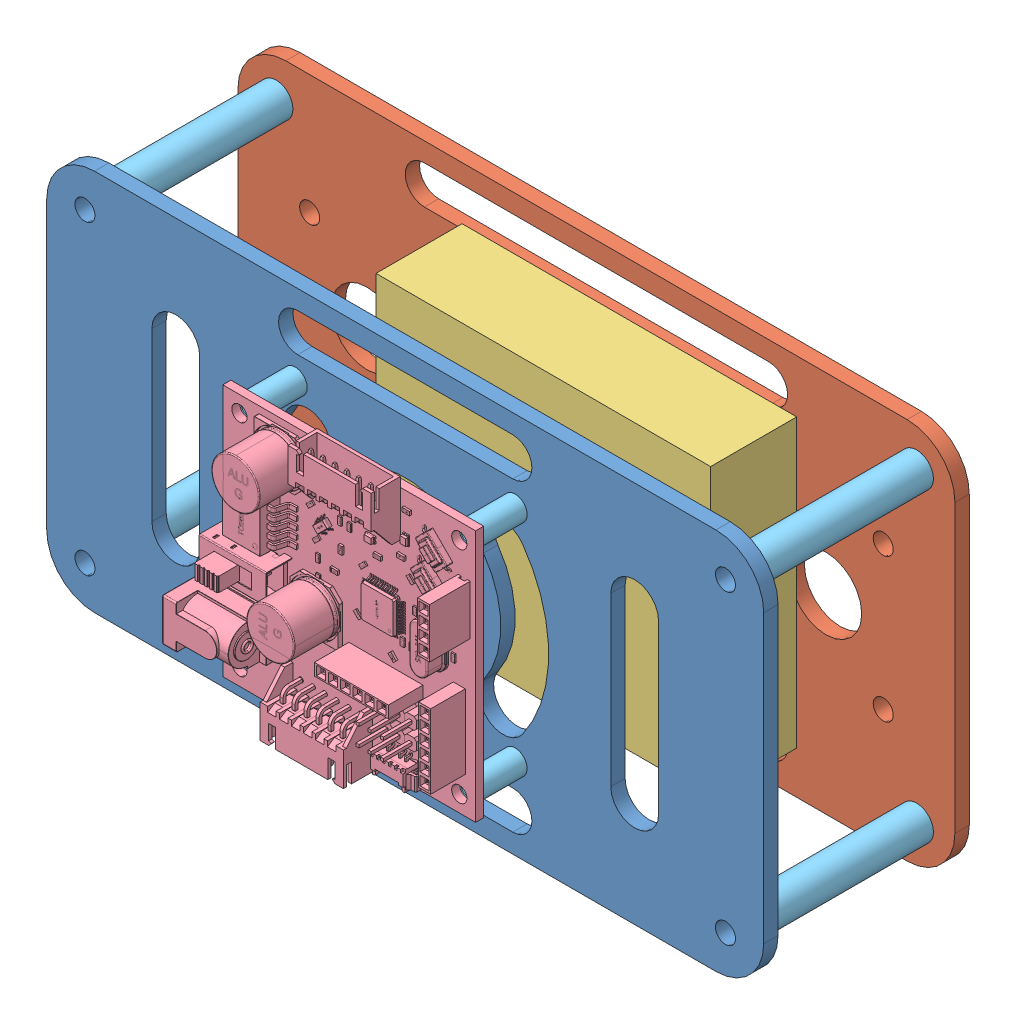
SolidWorks assembly 平衡车装配体, configuration 默认. Lengths in mm.
Overall size (150 80 69.68).
12 component instances, 5 part files, 23 mates.
Components (placement in the parent):
- 上层板-1: 上层板 [默认] at (-102.0399 47.0897 148.5) size (150 80 3)
- 下层板-1: 下层板 [默认] at (-102.0399 -32.9103 111.5) x (1 0 0) z (0 0 -1) size (150 80 3)
- 电池-1: 电池 [默认] at (-55.1505 36.0162 111.5) size (70 60 18)
- 平衡车驱动板-1: 平衡车驱动板 [默认] at (-101.0399 -60.9103 163.1914) size (54.74 56.4 19.75)
- 铝柱-2: 铝柱 [M4*37] at (39.9601 39.0897 130) x (1 0 0) z (0 1 0) size (7 37 7)
- 铝柱-3: 铝柱 [M4*37] at (-94.0399 -24.9103 130) x (-0.451929 0.892054 0) z (-0.892054 -0.451929 0) size (7 37 7)
- 铝柱-4: 铝柱 [M4*37] at (-94.0399 39.0897 130) x (1 0 0) z (0 1 0) size (7 37 7)
- 铝柱-5: 铝柱 [M4*37] at (39.9601 -24.9103 130) x (1 0 0) z (0 1 0) size (7 37 7)
- 铝柱-6: 铝柱 [M3*10] at (-4.0399 -15.9103 156.5) x (1 0 0) z (0 1 0) size (5 10 5)
- 铝柱-7: 铝柱 [M3*10] at (-4.0399 30.0897 156.5) x (1 0 0) z (0 1 0) size (5 10 5)
- 铝柱-8: 铝柱 [M3*10] at (-50.0399 30.0897 156.5) x (1 0 0) z (0 1 0) size (5 10 5)
- 铝柱-9: 铝柱 [M3*10] at (-50.0399 -15.9103 156.5) x (1 0 0) z (0 1 0) size (5 10 5)
Mates (geometry in assembly coordinates):
- 同心2: concentric anti-aligned: cylinder of 上层板-1 through (-94.0399 39.0897 151.5) axis (0 0 -1) radius 2.1; cylinder of 铝柱-4 through (-94.0399 39.0897 148.5) axis (0 0 1) radius 1.25
- 同心3: concentric aligned: circle of 上层板-1; circle of 铝柱-3
- 同心4: concentric anti-aligned: cylinder of 上层板-1 through (39.9601 -24.9103 151.5) axis (0 0 -1) radius 2.1; cylinder of 铝柱-5 through (39.9601 -24.9103 148.5) axis (0 0 1) radius 1.25
- 同心5: concentric anti-aligned: cylinder of 上层板-1 through (39.9601 39.0897 151.5) axis (0 0 -1) radius 2.1; cylinder of 铝柱-2 through (39.9601 39.0897 148.5) axis (0 0 1) radius 1.25
- 重合3: coincident anti-aligned: plane of 上层板-1 through (-92.0399 -22.9103 148.5) normal (0 0 -1); plane of 铝柱-4 through (-94.0399 39.0897 148.5) normal (0 0 1)
- 重合4: coincident anti-aligned: plane of 上层板-1 through (-92.0399 -22.9103 148.5) normal (0 0 -1); plane of 铝柱-3 through (-94.0399 -24.9103 148.5) normal (0 0 1)
- 重合5: coincident anti-aligned: plane of 上层板-1 through (-92.0399 -22.9103 148.5) normal (0 0 -1); plane of 铝柱-5 through (39.9601 -24.9103 148.5) normal (0 0 1)
- 重合6: coincident anti-aligned: plane of 上层板-1 through (-92.0399 -22.9103 148.5) normal (0 0 -1); plane of 铝柱-2 through (39.9601 39.0897 148.5) normal (0 0 1)
- 重合7: coincident anti-aligned: plane of 下层板-1 through (37.9601 -22.9103 111.5) normal (0 0 1); plane of 铝柱-2 through (39.9601 39.0897 111.5) normal (0 0 -1)
- 同心6: concentric anti-aligned: cylinder of 下层板-1 through (39.9601 39.0897 108.5) axis (0 0 1) radius 2.1; cylinder of 铝柱-2 through (39.9601 39.0897 111.5) axis (0 0 -1) radius 1.25
- 同心7: concentric anti-aligned: cylinder of 下层板-1 through (-94.0399 -24.9103 108.5) axis (0 0 1) radius 2.1; cylinder of 铝柱-3 through (-94.0399 -24.9103 111.5) axis (0 0 -1) radius 1.25
- 重合8: coincident anti-aligned: plane of 下层板-1 through (37.9601 -22.9103 111.5) normal (0 0 1); plane of 电池-1 through (-55.1505 36.0162 111.5) normal (0 0 -1)
- 同心81: concentric aligned: cylinder of 上层板-1 through (-4.0399 -15.9103 148.5) axis (0 0 1) radius 1.6; cylinder of 铝柱-6 through (-4.0399 -15.9103 151.5) axis (0 0 1) radius 2.5
- 重合91: coincident anti-aligned: plane of 上层板-1 through (-92.0399 -22.9103 151.5) normal (0 0 1); plane of 铝柱-6 through (-4.0399 -15.9103 151.5) normal (0 0 -1)
- 同心91: concentric aligned: cylinder of 上层板-1 through (-4.0399 30.0897 148.5) axis (0 0 1) radius 1.6; cylinder of 铝柱-7 through (-4.0399 30.0897 151.5) axis (0 0 1) radius 2.5
- 重合101: coincident anti-aligned: plane of 上层板-1 through (-92.0399 -22.9103 151.5) normal (0 0 1); plane of 铝柱-7 through (-4.0399 30.0897 151.5) normal (0 0 -1)
- 同心101: concentric aligned: cylinder of 上层板-1 through (-50.0399 30.0897 148.5) axis (0 0 1) radius 1.6; cylinder of 铝柱-8 through (-50.0399 30.0897 151.5) axis (0 0 1) radius 2.5
- 重合111: coincident anti-aligned: plane of 上层板-1 through (-92.0399 -22.9103 151.5) normal (0 0 1); plane of 铝柱-8 through (-50.0399 30.0897 151.5) normal (0 0 -1)
- 同心111: concentric aligned: cylinder of 上层板-1 through (-50.0399 -15.9103 148.5) axis (0 0 1) radius 1.6; cylinder of 铝柱-9 through (-50.0399 -15.9103 151.5) axis (0 0 1) radius 2.5
- 重合121: coincident anti-aligned: plane of 上层板-1 through (-92.0399 -22.9103 151.5) normal (0 0 1); plane of 铝柱-9 through (-50.0399 -15.9103 151.5) normal (0 0 -1)
- 同心12: concentric anti-aligned: cylinder of 平衡车驱动板-1 through (-4.0399 -15.9103 161.5) axis (0 0 -1) radius 1.6; cylinder of 铝柱-6 through (-4.0399 -15.9103 161.5) axis (0 0 1) radius 1.25
- 同心13: concentric anti-aligned: cylinder of 平衡车驱动板-1 through (-50.0399 -15.9103 161.5) axis (0 0 -1) radius 1.6; cylinder of 铝柱-9 through (-50.0399 -15.9103 161.5) axis (0 0 1) radius 1.25
- 重合13: coincident anti-aligned: plane of 平衡车驱动板-1 through (-53.5149 -19.3853 161.5) normal (0 0 -1); plane of 铝柱-9 through (-50.0399 -15.9103 161.5) normal (0 0 1)
